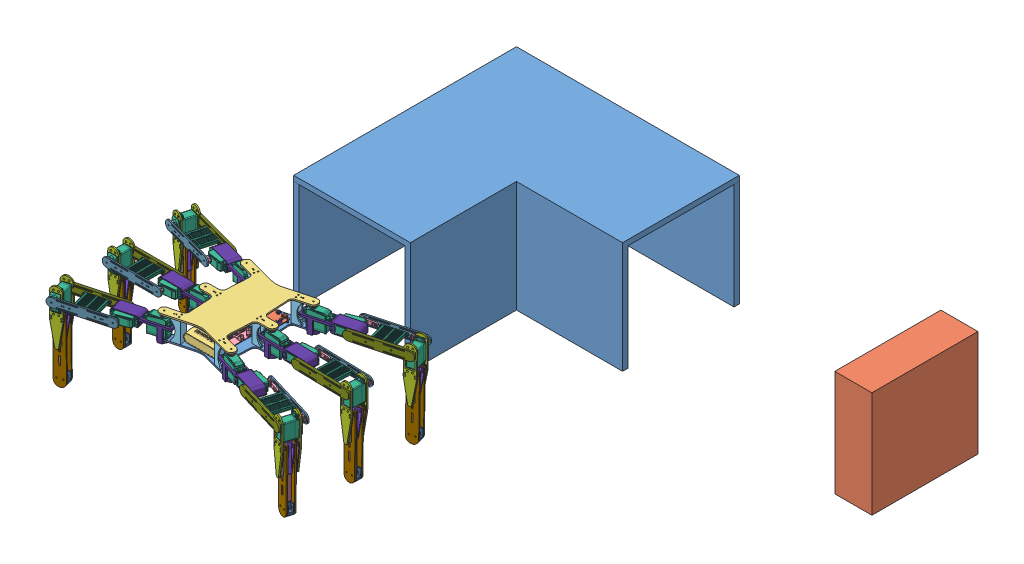
SolidWorks assembly ObstacleCourse, configuration Default. Lengths in mm.
Overall size (1281.29 282.9 1001.36).
210 component instances, 40 part files, 3 mates.
Components (placement in the parent):
- Tunnel-1: Tunnel [Default] at (-133.9096 207.5789 158.7477) x (0 0 1) z (-1 0 0) size (533.4 266.7 533.4)
- Wall-1: Wall [Default] at (894.7904 207.5789 425.4477) size (88.9 254 254)
- FullAssembly-1: FullAssembly [Default] at (-185.9141 155.1575 649.3406) size (590.09 222.09 384.76)
  - BodyAssembly-1: BodyAssembly [Default] at (93.0903 134.9257 147.182) size (181 51.83 218.31)
    - TopPlate-1: TopPlate [Default] at (90.5661 120.22 158.5049) size (181 3.17 218.31)
    - Aluminium 25T Servo Horn-1: Aluminium 25T Servo Horn [Default] at (10.5661 120.22 257.1595) x (0.965926 0 -0.258819) z (0 1 0) size (35.39 15.87 6)
    - Aluminium 25T Servo Horn-2: Aluminium 25T Servo Horn [Default] at (10.5661 120.22 158.5049) x (1 0 0) z (0 1 0) size (35.39 15.87 6)
    - Aluminium 25T Servo Horn-3: Aluminium 25T Servo Horn [Default] at (170.5661 120.22 257.1595) x (-0.965926 0 -0.258819) z (0 1 0) size (35.39 15.87 6)
    - Aluminium 25T Servo Horn-4: Aluminium 25T Servo Horn [Default] at (170.5661 120.22 59.8503) x (-0.965926 0 0.258819) z (0 1 0) size (35.39 15.87 6)
    - Aluminium 25T Servo Horn-5: Aluminium 25T Servo Horn [Default] at (170.5661 120.22 158.5049) x (-1 0 0) z (0 1 0) size (35.39 15.87 6)
    - Aluminium 25T Servo Horn-6: Aluminium 25T Servo Horn [Default] at (10.5661 120.22 59.8503) x (0.965926 0 0.258819) z (0 1 0) size (35.39 15.87 6)
    - BodyStandoff-1: BodyStandoff [Default] at (155.8504 117.045 74.4774) x (-0.965926 0 0.258819) z (0 -1 0) size (20 20.64 48.65)
    - BodyStandoff-2: BodyStandoff [Default] at (28.5661 117.045 148.1849) x (1 0 0) z (0 -1 0) size (20 20.64 48.65)
    - BodyStandoff-3: BodyStandoff [Default] at (152.5661 117.045 168.8249) x (-1 0 0) z (0 -1 0) size (20 20.64 48.65)
    - BodyStandoff-4: BodyStandoff [Default] at (150.5084 117.045 262.4691) x (-0.965926 0 -0.258819) z (0 -1 0) size (20 20.64 48.65)
    - BodyStandoff-5: BodyStandoff [Default] at (30.6238 117.045 54.5407) x (0.965926 0 0.258819) z (0 -1 0) size (20 20.64 48.65)
    - BodyStandoff-6: BodyStandoff [Default] at (25.2817 117.045 242.5324) x (0.965926 0 -0.258819) z (0 -1 0) size (20 20.64 48.65)
  - LegAssembly-1: LegAssembly [Default] at (68.7155 20.3576 359.6903) x (0.267323 -0.008627 0.963568) z (-0.963568 -0.011394 0.267221) size (60.68 215.89 234.68)
    - LowerLegAssembly-1: LowerLegAssembly [Default] at (27.0721 179.3541 216.2254) x (-0.008726 0.999962 -0.000076) z (0.008727 0 -0.999962) size (214.1 48.83 26)
      - 20kg Servo-1: 20kg Servo [Default] at (19.931 7.4761 41.5788) size (55.1 45.65 20.12)
      - KneeFrontPlate-1: KneeFrontPlate [Default] at (40.481 40.4761 41.5788) x (0 0 1) z (-1 0 0) size (26 3.17 130.1)
      - KneeFrontPlate-2: KneeFrontPlate [Default] at (40.481 4.3011 41.5788) x (0 0 1) z (-1 0 0) size (26 3.17 130.1)
      - LowerLegMiddleStandoff-1: LowerLegMiddleStandoff [Default] at (-7.619 28.6386 34.2851) x (0 0 1) z (-1 0 0) size (11.41 13.32 68)
      - LowerLegMiddleStandoff-2: LowerLegMiddleStandoff [Default] at (-7.619 19.3136 48.8726) x (0 0 -1) z (-1 0 0) size (11.41 13.32 68)
      - LowerLegPlate-1: LowerLegPlate [Default] at (-7.619 30.6386 43.1663) x (0 0 1) z (-1 0 0) size (26 3.17 153)
      - LowerLegPlate-2: LowerLegPlate [Default] at (-7.619 14.1386 43.1663) x (0 0 1) z (-1 0 0) size (26 3.17 153)
      - Foot-1: Foot [Default] at (-142.619 28.6436 41.5788) x (0 0 1) z (-1 0 0) size (26 13.33 28)
      - LowerLegSideStandoff-1: LowerLegSideStandoff [Default] at (-7.619 38.4761 34.2851) x (0 0 1) z (-1 0 0) size (11.41 6.66 68)
      - LowerLegSideStandoff-4: LowerLegSideStandoff [Default] at (-7.619 9.4761 48.8726) x (0 0 -1) z (-1 0 0) size (11.41 6.66 68)
      - MirrorLowerLegSideStandoff-10: MirrorLowerLegSideStandoff [Default] at (-7.619 9.4761 34.2851) x (0 0 1) z (1 0 0) size (11.41 6.66 68)
      - MirrorLowerLegSideStandoff-11: MirrorLowerLegSideStandoff [Default] at (-7.619 38.4761 48.8726) x (0 0 -1) z (1 0 0) size (11.41 6.66 68)
      - LowerLegBone-1: LowerLegBone [Default] at (-7.619 23.9761 43.1663) x (0 1 0) z (-1 0 0) size (33 3.17 135)
    - UpperLegAssembly-1: UpperLegAssembly [Default] at (52.8994 191.2742 177.6224) x (0.008825 -0.011318 -0.999897) z (0.999924 0.008727 0.008726) size (231.45 53.65 58.17)
      - Aluminium 25T Servo Horn-1: Aluminium 25T Servo Horn [Default] at (2.5459 18.2137 30.5337) size (35.39 15.87 6)
      - UpperLegFront-1: UpperLegFront [Default] at (2.5459 18.2137 33.7087) x (0 -1 0) z (1 0 0) size (21 3.17 141)
      - Aluminium 25T Servo Horn-2: Aluminium 25T Servo Horn [Default] at (122.5459 18.2137 30.5337) x (-1 0 0) z (0 0 1) size (35.39 15.87 6)
      - 20kg Servo-1: 20kg Servo [Default] at (132.4959 18.2137 -18.1163) x (-1 0 0) z (0 1 0) size (55.1 45.65 20.12)
      - UpperLegStandoff-1: UpperLegStandoff [Default] at (37.6959 18.2137 -18.1163) x (0 1 0) z (1 0 0) size (6 48.65 56)
      - UpperLegBack-1: UpperLegBack [Default] at (2.5459 18.2137 -18.1163) x (0 -1 0) z (1 0 0) size (21 3.17 141)
      - ShoulderMount-1: ShoulderMount [Default] at (102.5459 27.8363 -18.1163) x (1 0 0) z (0 -1 0) size (120 28.35 40.35)
      - 20kg Servo-2: 20kg Servo [Default] at (191.5459 -2.6363 -3.9413) size (55.1 45.65 20.12)
      - UpperLegBack-2: UpperLegBack [Default] at (2.5459 18.2137 -21.2913) x (0 -1 0) z (1 0 0) size (21 3.17 141)
    - Bearing-1: Bearing [Default] at (50.8194 178.3353 -22.7661) x (-0.059991 -0.011892 -0.998128) z (0.998162 0.007927 -0.060087) size (16 5 16)
  - LegAssembly-2: LegAssembly [Default] at (81.4626 20.3576 253.5138) x (0.008825 -0.008627 0.999924) z (-0.999897 -0.011394 0.008726) size (60.68 215.89 234.68)
    - LowerLegAssembly-1: LowerLegAssembly [Default] at (27.0721 179.3541 216.2254) x (-0.008726 0.999962 -0.000076) z (0.008727 0 -0.999962) size (214.1 48.83 26)
      - 20kg Servo-1: 20kg Servo [Default] at (19.931 7.4761 41.5788) size (55.1 45.65 20.12)
      - KneeFrontPlate-1: KneeFrontPlate [Default] at (40.481 40.4761 41.5788) x (0 0 1) z (-1 0 0) size (26 3.17 130.1)
      - KneeFrontPlate-2: KneeFrontPlate [Default] at (40.481 4.3011 41.5788) x (0 0 1) z (-1 0 0) size (26 3.17 130.1)
      - LowerLegMiddleStandoff-1: LowerLegMiddleStandoff [Default] at (-7.619 28.6386 34.2851) x (0 0 1) z (-1 0 0) size (11.41 13.32 68)
      - LowerLegMiddleStandoff-2: LowerLegMiddleStandoff [Default] at (-7.619 19.3136 48.8726) x (0 0 -1) z (-1 0 0) size (11.41 13.32 68)
      - LowerLegPlate-1: LowerLegPlate [Default] at (-7.619 30.6386 43.1663) x (0 0 1) z (-1 0 0) size (26 3.17 153)
      - LowerLegPlate-2: LowerLegPlate [Default] at (-7.619 14.1386 43.1663) x (0 0 1) z (-1 0 0) size (26 3.17 153)
      - Foot-1: Foot [Default] at (-142.619 28.6436 41.5788) x (0 0 1) z (-1 0 0) size (26 13.33 28)
      - LowerLegSideStandoff-1: LowerLegSideStandoff [Default] at (-7.619 38.4761 34.2851) x (0 0 1) z (-1 0 0) size (11.41 6.66 68)
      - LowerLegSideStandoff-4: LowerLegSideStandoff [Default] at (-7.619 9.4761 48.8726) x (0 0 -1) z (-1 0 0) size (11.41 6.66 68)
      - MirrorLowerLegSideStandoff-10: MirrorLowerLegSideStandoff [Default] at (-7.619 9.4761 34.2851) x (0 0 1) z (1 0 0) size (11.41 6.66 68)
      - MirrorLowerLegSideStandoff-11: MirrorLowerLegSideStandoff [Default] at (-7.619 38.4761 48.8726) x (0 0 -1) z (1 0 0) size (11.41 6.66 68)
      - LowerLegBone-1: LowerLegBone [Default] at (-7.619 23.9761 43.1663) x (0 1 0) z (-1 0 0) size (33 3.17 135)
    - UpperLegAssembly-1: UpperLegAssembly [Default] at (52.8994 191.2742 177.6224) x (0.008825 -0.011318 -0.999897) z (0.999924 0.008727 0.008726) size (231.45 53.65 58.17)
      - Aluminium 25T Servo Horn-1: Aluminium 25T Servo Horn [Default] at (2.5459 18.2137 30.5337) size (35.39 15.87 6)
      - UpperLegFront-1: UpperLegFront [Default] at (2.5459 18.2137 33.7087) x (0 -1 0) z (1 0 0) size (21 3.17 141)
      - Aluminium 25T Servo Horn-2: Aluminium 25T Servo Horn [Default] at (122.5459 18.2137 30.5337) x (-1 0 0) z (0 0 1) size (35.39 15.87 6)
      - 20kg Servo-1: 20kg Servo [Default] at (132.4959 18.2137 -18.1163) x (-1 0 0) z (0 1 0) size (55.1 45.65 20.12)
      - UpperLegStandoff-1: UpperLegStandoff [Default] at (37.6959 18.2137 -18.1163) x (0 1 0) z (1 0 0) size (6 48.65 56)
      - UpperLegBack-1: UpperLegBack [Default] at (2.5459 18.2137 -18.1163) x (0 -1 0) z (1 0 0) size (21 3.17 141)
      - ShoulderMount-1: ShoulderMount [Default] at (102.5459 27.8363 -18.1163) x (1 0 0) z (0 -1 0) size (120 28.35 40.35)
      - 20kg Servo-2: 20kg Servo [Default] at (191.5459 -2.6363 -3.9413) size (55.1 45.65 20.12)
      - UpperLegBack-2: UpperLegBack [Default] at (2.5459 18.2137 -21.2913) x (0 -1 0) z (1 0 0) size (21 3.17 141)
    - Bearing-1: Bearing [Default] at (50.8194 178.3353 -22.7661) x (-0.059991 -0.011892 -0.998128) z (0.998162 0.007927 -0.060087) size (16 5 16)
  - LegAssembly-3: LegAssembly [Default] at (95.7223 20.3576 150.8928) x (-0.250275 -0.008627 0.968136) z (-0.968085 -0.011394 -0.250364) size (60.68 215.89 234.68)
    - LowerLegAssembly-1: LowerLegAssembly [Default] at (27.0721 179.3541 216.2254) x (-0.008726 0.999962 -0.000076) z (0.008727 0 -0.999962) size (214.1 48.83 26)
      - 20kg Servo-1: 20kg Servo [Default] at (19.931 7.4761 41.5788) size (55.1 45.65 20.12)
      - KneeFrontPlate-1: KneeFrontPlate [Default] at (40.481 40.4761 41.5788) x (0 0 1) z (-1 0 0) size (26 3.17 130.1)
      - KneeFrontPlate-2: KneeFrontPlate [Default] at (40.481 4.3011 41.5788) x (0 0 1) z (-1 0 0) size (26 3.17 130.1)
      - LowerLegMiddleStandoff-1: LowerLegMiddleStandoff [Default] at (-7.619 28.6386 34.2851) x (0 0 1) z (-1 0 0) size (11.41 13.32 68)
      - LowerLegMiddleStandoff-2: LowerLegMiddleStandoff [Default] at (-7.619 19.3136 48.8726) x (0 0 -1) z (-1 0 0) size (11.41 13.32 68)
      - LowerLegPlate-1: LowerLegPlate [Default] at (-7.619 30.6386 43.1663) x (0 0 1) z (-1 0 0) size (26 3.17 153)
      - LowerLegPlate-2: LowerLegPlate [Default] at (-7.619 14.1386 43.1663) x (0 0 1) z (-1 0 0) size (26 3.17 153)
      - Foot-1: Foot [Default] at (-142.619 28.6436 41.5788) x (0 0 1) z (-1 0 0) size (26 13.33 28)
      - LowerLegSideStandoff-1: LowerLegSideStandoff [Default] at (-7.619 38.4761 34.2851) x (0 0 1) z (-1 0 0) size (11.41 6.66 68)
      - LowerLegSideStandoff-4: LowerLegSideStandoff [Default] at (-7.619 9.4761 48.8726) x (0 0 -1) z (-1 0 0) size (11.41 6.66 68)
      - MirrorLowerLegSideStandoff-10: MirrorLowerLegSideStandoff [Default] at (-7.619 9.4761 34.2851) x (0 0 1) z (1 0 0) size (11.41 6.66 68)
      - MirrorLowerLegSideStandoff-11: MirrorLowerLegSideStandoff [Default] at (-7.619 38.4761 48.8726) x (0 0 -1) z (1 0 0) size (11.41 6.66 68)
      - LowerLegBone-1: LowerLegBone [Default] at (-7.619 23.9761 43.1663) x (0 1 0) z (-1 0 0) size (33 3.17 135)
    - UpperLegAssembly-1: UpperLegAssembly [Default] at (52.8994 191.2742 177.6224) x (0.008825 -0.011318 -0.999897) z (0.999924 0.008727 0.008726) size (231.45 53.65 58.17)
      - Aluminium 25T Servo Horn-1: Aluminium 25T Servo Horn [Default] at (2.5459 18.2137 30.5337) size (35.39 15.87 6)
      - UpperLegFront-1: UpperLegFront [Default] at (2.5459 18.2137 33.7087) x (0 -1 0) z (1 0 0) size (21 3.17 141)
      - Aluminium 25T Servo Horn-2: Aluminium 25T Servo Horn [Default] at (122.5459 18.2137 30.5337) x (-1 0 0) z (0 0 1) size (35.39 15.87 6)
      - 20kg Servo-1: 20kg Servo [Default] at (132.4959 18.2137 -18.1163) x (-1 0 0) z (0 1 0) size (55.1 45.65 20.12)
      - UpperLegStandoff-1: UpperLegStandoff [Default] at (37.6959 18.2137 -18.1163) x (0 1 0) z (1 0 0) size (6 48.65 56)
      - UpperLegBack-1: UpperLegBack [Default] at (2.5459 18.2137 -18.1163) x (0 -1 0) z (1 0 0) size (21 3.17 141)
      - ShoulderMount-1: ShoulderMount [Default] at (102.5459 27.8363 -18.1163) x (1 0 0) z (0 -1 0) size (120 28.35 40.35)
      - 20kg Servo-2: 20kg Servo [Default] at (191.5459 -2.6363 -3.9413) size (55.1 45.65 20.12)
      - UpperLegBack-2: UpperLegBack [Default] at (2.5459 18.2137 -21.2913) x (0 -1 0) z (1 0 0) size (21 3.17 141)
    - Bearing-1: Bearing [Default] at (50.8194 178.3353 -22.7661) x (-0.059991 -0.011892 -0.998128) z (0.998162 0.007927 -0.060087) size (16 5 16)
  - LegAssembly-4: LegAssembly [Default] at (269.8625 20.3576 460.6982) x (0.279891 -0.008627 -0.959993) z (0.959939 -0.011394 0.279977) size (60.68 215.89 234.68)
    - LowerLegAssembly-1: LowerLegAssembly [Default] at (27.0721 179.3541 216.2254) x (-0.008726 0.999962 -0.000076) z (0.008727 0 -0.999962) size (214.1 48.83 26)
      - 20kg Servo-1: 20kg Servo [Default] at (19.931 7.4761 41.5788) size (55.1 45.65 20.12)
      - KneeFrontPlate-1: KneeFrontPlate [Default] at (40.481 40.4761 41.5788) x (0 0 1) z (-1 0 0) size (26 3.17 130.1)
      - KneeFrontPlate-2: KneeFrontPlate [Default] at (40.481 4.3011 41.5788) x (0 0 1) z (-1 0 0) size (26 3.17 130.1)
      - LowerLegMiddleStandoff-1: LowerLegMiddleStandoff [Default] at (-7.619 28.6386 34.2851) x (0 0 1) z (-1 0 0) size (11.41 13.32 68)
      - LowerLegMiddleStandoff-2: LowerLegMiddleStandoff [Default] at (-7.619 19.3136 48.8726) x (0 0 -1) z (-1 0 0) size (11.41 13.32 68)
      - LowerLegPlate-1: LowerLegPlate [Default] at (-7.619 30.6386 43.1663) x (0 0 1) z (-1 0 0) size (26 3.17 153)
      - LowerLegPlate-2: LowerLegPlate [Default] at (-7.619 14.1386 43.1663) x (0 0 1) z (-1 0 0) size (26 3.17 153)
      - Foot-1: Foot [Default] at (-142.619 28.6436 41.5788) x (0 0 1) z (-1 0 0) size (26 13.33 28)
      - LowerLegSideStandoff-1: LowerLegSideStandoff [Default] at (-7.619 38.4761 34.2851) x (0 0 1) z (-1 0 0) size (11.41 6.66 68)
      - LowerLegSideStandoff-4: LowerLegSideStandoff [Default] at (-7.619 9.4761 48.8726) x (0 0 -1) z (-1 0 0) size (11.41 6.66 68)
      - MirrorLowerLegSideStandoff-10: MirrorLowerLegSideStandoff [Default] at (-7.619 9.4761 34.2851) x (0 0 1) z (1 0 0) size (11.41 6.66 68)
      - MirrorLowerLegSideStandoff-11: MirrorLowerLegSideStandoff [Default] at (-7.619 38.4761 48.8726) x (0 0 -1) z (1 0 0) size (11.41 6.66 68)
      - LowerLegBone-1: LowerLegBone [Default] at (-7.619 23.9761 43.1663) x (0 1 0) z (-1 0 0) size (33 3.17 135)
    - UpperLegAssembly-1: UpperLegAssembly [Default] at (52.8994 191.2742 177.6224) x (0.008825 -0.011318 -0.999897) z (0.999924 0.008727 0.008726) size (231.45 53.65 58.17)
      - Aluminium 25T Servo Horn-1: Aluminium 25T Servo Horn [Default] at (2.5459 18.2137 30.5337) size (35.39 15.87 6)
      - UpperLegFront-1: UpperLegFront [Default] at (2.5459 18.2137 33.7087) x (0 -1 0) z (1 0 0) size (21 3.17 141)
      - Aluminium 25T Servo Horn-2: Aluminium 25T Servo Horn [Default] at (122.5459 18.2137 30.5337) x (-1 0 0) z (0 0 1) size (35.39 15.87 6)
      - 20kg Servo-1: 20kg Servo [Default] at (132.4959 18.2137 -18.1163) x (-1 0 0) z (0 1 0) size (55.1 45.65 20.12)
      - UpperLegStandoff-1: UpperLegStandoff [Default] at (37.6959 18.2137 -18.1163) x (0 1 0) z (1 0 0) size (6 48.65 56)
      - UpperLegBack-1: UpperLegBack [Default] at (2.5459 18.2137 -18.1163) x (0 -1 0) z (1 0 0) size (21 3.17 141)
      - ShoulderMount-1: ShoulderMount [Default] at (102.5459 27.8363 -18.1163) x (1 0 0) z (0 -1 0) size (120 28.35 40.35)
      - 20kg Servo-2: 20kg Servo [Default] at (191.5459 -2.6363 -3.9413) size (55.1 45.65 20.12)
      - UpperLegBack-2: UpperLegBack [Default] at (2.5459 18.2137 -21.2913) x (0 -1 0) z (1 0 0) size (21 3.17 141)
    - Bearing-1: Bearing [Default] at (50.8194 178.3353 -22.7661) x (-0.059991 -0.011892 -0.998128) z (0.998162 0.007927 -0.060087) size (16 5 16)
  - LegAssembly-5: LegAssembly [Default] at (284.5268 20.3576 358.4033) x (0.016403 -0.008627 -0.999828) z (0.999799 -0.011394 0.016501) size (60.68 215.89 234.68)
    - LowerLegAssembly-1: LowerLegAssembly [Default] at (27.0721 179.3541 216.2254) x (-0.008726 0.999962 -0.000076) z (0.008727 0 -0.999962) size (214.1 48.83 26)
      - 20kg Servo-1: 20kg Servo [Default] at (19.931 7.4761 41.5788) size (55.1 45.65 20.12)
      - KneeFrontPlate-1: KneeFrontPlate [Default] at (40.481 40.4761 41.5788) x (0 0 1) z (-1 0 0) size (26 3.17 130.1)
      - KneeFrontPlate-2: KneeFrontPlate [Default] at (40.481 4.3011 41.5788) x (0 0 1) z (-1 0 0) size (26 3.17 130.1)
      - LowerLegMiddleStandoff-1: LowerLegMiddleStandoff [Default] at (-7.619 28.6386 34.2851) x (0 0 1) z (-1 0 0) size (11.41 13.32 68)
      - LowerLegMiddleStandoff-2: LowerLegMiddleStandoff [Default] at (-7.619 19.3136 48.8726) x (0 0 -1) z (-1 0 0) size (11.41 13.32 68)
      - LowerLegPlate-1: LowerLegPlate [Default] at (-7.619 30.6386 43.1663) x (0 0 1) z (-1 0 0) size (26 3.17 153)
      - LowerLegPlate-2: LowerLegPlate [Default] at (-7.619 14.1386 43.1663) x (0 0 1) z (-1 0 0) size (26 3.17 153)
      - Foot-1: Foot [Default] at (-142.619 28.6436 41.5788) x (0 0 1) z (-1 0 0) size (26 13.33 28)
      - LowerLegSideStandoff-1: LowerLegSideStandoff [Default] at (-7.619 38.4761 34.2851) x (0 0 1) z (-1 0 0) size (11.41 6.66 68)
      - LowerLegSideStandoff-4: LowerLegSideStandoff [Default] at (-7.619 9.4761 48.8726) x (0 0 -1) z (-1 0 0) size (11.41 6.66 68)
      - MirrorLowerLegSideStandoff-10: MirrorLowerLegSideStandoff [Default] at (-7.619 9.4761 34.2851) x (0 0 1) z (1 0 0) size (11.41 6.66 68)
      - MirrorLowerLegSideStandoff-11: MirrorLowerLegSideStandoff [Default] at (-7.619 38.4761 48.8726) x (0 0 -1) z (1 0 0) size (11.41 6.66 68)
      - LowerLegBone-1: LowerLegBone [Default] at (-7.619 23.9761 43.1663) x (0 1 0) z (-1 0 0) size (33 3.17 135)
    - UpperLegAssembly-1: UpperLegAssembly [Default] at (52.8994 191.2742 177.6224) x (0.008825 -0.011318 -0.999897) z (0.999924 0.008727 0.008726) size (231.45 53.65 58.17)
      - Aluminium 25T Servo Horn-1: Aluminium 25T Servo Horn [Default] at (2.5459 18.2137 30.5337) size (35.39 15.87 6)
      - UpperLegFront-1: UpperLegFront [Default] at (2.5459 18.2137 33.7087) x (0 -1 0) z (1 0 0) size (21 3.17 141)
      - Aluminium 25T Servo Horn-2: Aluminium 25T Servo Horn [Default] at (122.5459 18.2137 30.5337) x (-1 0 0) z (0 0 1) size (35.39 15.87 6)
      - 20kg Servo-1: 20kg Servo [Default] at (132.4959 18.2137 -18.1163) x (-1 0 0) z (0 1 0) size (55.1 45.65 20.12)
      - UpperLegStandoff-1: UpperLegStandoff [Default] at (37.6959 18.2137 -18.1163) x (0 1 0) z (1 0 0) size (6 48.65 56)
      - UpperLegBack-1: UpperLegBack [Default] at (2.5459 18.2137 -18.1163) x (0 -1 0) z (1 0 0) size (21 3.17 141)
      - ShoulderMount-1: ShoulderMount [Default] at (102.5459 27.8363 -18.1163) x (1 0 0) z (0 -1 0) size (120 28.35 40.35)
      - 20kg Servo-2: 20kg Servo [Default] at (191.5459 -2.6363 -3.9413) size (55.1 45.65 20.12)
      - UpperLegBack-2: UpperLegBack [Default] at (2.5459 18.2137 -21.2913) x (0 -1 0) z (1 0 0) size (21 3.17 141)
    - Bearing-1: Bearing [Default] at (50.8194 178.3353 -22.7661) x (-0.059991 -0.011892 -0.998128) z (0.998162 0.007927 -0.060087) size (16 5 16)
  - LegAssembly-6: LegAssembly [Default] at (298.5972 20.3576 251.6835) x (-0.267323 -0.008627 -0.963568) z (0.963568 -0.011394 -0.267221) size (60.68 215.89 234.68)
    - LowerLegAssembly-1: LowerLegAssembly [Default] at (27.0721 179.3541 216.2254) x (-0.008726 0.999962 -0.000076) z (0.008727 0 -0.999962) size (214.1 48.83 26)
      - 20kg Servo-1: 20kg Servo [Default] at (19.931 7.4761 41.5788) size (55.1 45.65 20.12)
      - KneeFrontPlate-1: KneeFrontPlate [Default] at (40.481 40.4761 41.5788) x (0 0 1) z (-1 0 0) size (26 3.17 130.1)
      - KneeFrontPlate-2: KneeFrontPlate [Default] at (40.481 4.3011 41.5788) x (0 0 1) z (-1 0 0) size (26 3.17 130.1)
      - LowerLegMiddleStandoff-1: LowerLegMiddleStandoff [Default] at (-7.619 28.6386 34.2851) x (0 0 1) z (-1 0 0) size (11.41 13.32 68)
      - LowerLegMiddleStandoff-2: LowerLegMiddleStandoff [Default] at (-7.619 19.3136 48.8726) x (0 0 -1) z (-1 0 0) size (11.41 13.32 68)
      - LowerLegPlate-1: LowerLegPlate [Default] at (-7.619 30.6386 43.1663) x (0 0 1) z (-1 0 0) size (26 3.17 153)
      - LowerLegPlate-2: LowerLegPlate [Default] at (-7.619 14.1386 43.1663) x (0 0 1) z (-1 0 0) size (26 3.17 153)
      - Foot-1: Foot [Default] at (-142.619 28.6436 41.5788) x (0 0 1) z (-1 0 0) size (26 13.33 28)
      - LowerLegSideStandoff-1: LowerLegSideStandoff [Default] at (-7.619 38.4761 34.2851) x (0 0 1) z (-1 0 0) size (11.41 6.66 68)
      - LowerLegSideStandoff-4: LowerLegSideStandoff [Default] at (-7.619 9.4761 48.8726) x (0 0 -1) z (-1 0 0) size (11.41 6.66 68)
      - MirrorLowerLegSideStandoff-10: MirrorLowerLegSideStandoff [Default] at (-7.619 9.4761 34.2851) x (0 0 1) z (1 0 0) size (11.41 6.66 68)
      - MirrorLowerLegSideStandoff-11: MirrorLowerLegSideStandoff [Default] at (-7.619 38.4761 48.8726) x (0 0 -1) z (1 0 0) size (11.41 6.66 68)
      - LowerLegBone-1: LowerLegBone [Default] at (-7.619 23.9761 43.1663) x (0 1 0) z (-1 0 0) size (33 3.17 135)
    - UpperLegAssembly-1: UpperLegAssembly [Default] at (52.8994 191.2742 177.6224) x (0.008825 -0.011318 -0.999897) z (0.999924 0.008727 0.008726) size (231.45 53.65 58.17)
      - Aluminium 25T Servo Horn-1: Aluminium 25T Servo Horn [Default] at (2.5459 18.2137 30.5337) size (35.39 15.87 6)
      - UpperLegFront-1: UpperLegFront [Default] at (2.5459 18.2137 33.7087) x (0 -1 0) z (1 0 0) size (21 3.17 141)
      - Aluminium 25T Servo Horn-2: Aluminium 25T Servo Horn [Default] at (122.5459 18.2137 30.5337) x (-1 0 0) z (0 0 1) size (35.39 15.87 6)
      - 20kg Servo-1: 20kg Servo [Default] at (132.4959 18.2137 -18.1163) x (-1 0 0) z (0 1 0) size (55.1 45.65 20.12)
      - UpperLegStandoff-1: UpperLegStandoff [Default] at (37.6959 18.2137 -18.1163) x (0 1 0) z (1 0 0) size (6 48.65 56)
      - UpperLegBack-1: UpperLegBack [Default] at (2.5459 18.2137 -18.1163) x (0 -1 0) z (1 0 0) size (21 3.17 141)
      - ShoulderMount-1: ShoulderMount [Default] at (102.5459 27.8363 -18.1163) x (1 0 0) z (0 -1 0) size (120 28.35 40.35)
      - 20kg Servo-2: 20kg Servo [Default] at (191.5459 -2.6363 -3.9413) size (55.1 45.65 20.12)
      - UpperLegBack-2: UpperLegBack [Default] at (2.5459 18.2137 -21.2913) x (0 -1 0) z (1 0 0) size (21 3.17 141)
    - Bearing-1: Bearing [Default] at (50.8194 178.3353 -22.7661) x (-0.059991 -0.011892 -0.998128) z (0.998162 0.007927 -0.060087) size (16 5 16)
  - BottomBodyAssembly-1: BottomBodyAssembly [Default] at (83.95 98.1347 141.7913) size (181 28.22 218.31)
    - BottomPlate-1: BottomPlate [Default] at (99.7063 105.186 163.8956) size (181 3.17 218.31)
    - Raspberry Pi 4 Model B-1: Raspberry Pi 4 Model B [Default] at (101.4563 115.161 112.7766) x (-1 0 0) z (0 0 -1) size (88.99 19.9 58.4)
      - PCB, RPi4ModelB-1: PCB, RPi4ModelB [Default] at origin size (85 1.6 56)
      - Broadcom BCM2711B0 CPU, RPi4ModelB-1: Broadcom BCM2711B0 CPU, RPi4ModelB [Default] at (-13.25 0.8 -4.5) size (15 2.3 15)
      - 2.54 mm DUPONT MALE PIN HEADER, POE, 2X2, RPi4ModelB-1: 2.54 mm DUPONT MALE PIN HEADER, POE, 2X2, RPi4ModelB [Default] at (19 0.8 -18.5) size (5.08 11.3 5.08)
      - 2.54 mm DUPONT MALE PIN HEADER, IO, 2X20, RPi4ModelB-1: 2.54 mm DUPONT MALE PIN HEADER, IO, 2X20, RPi4ModelB [Default] at (-10 0.8 -24.5) size (50.8 11.3 5.08)
      - Camera Connector, RPi4ModelB-1: Camera Connector, RPi4ModelB [Default] at (4 0.8 16.5) x (0 0 -1) z (1 0 0) size (22.4 5.68 5.07)
      - Microphone Plug, RPi4ModelB-1: Microphone Plug, RPi4ModelB [Default] at (11.5 0.8 21.65) size (7.23 7.55 15)
      - Display Connector, RPi4ModelB-1: Display Connector, RPi4ModelB [Default] at (-38.5 0.8 0) x (0 0 1) z (-1 0 0) size (22.4 5.68 5.07)
      - Gigabit Ethernet Port, RPi4ModelB-1: Gigabit Ethernet Port, RPi4ModelB [Default] at (45.5 7.55 -17.75) x (0 0 -1) z (1 0 0) size (16.2 17.24 21.64)
      - Female Micro HDMI Connector, RPi4ModelB-2: Female Micro HDMI Connector, RPi4ModelB [Default] at (-3 0.8 27.3875) size (6.5 3.51 7.5)
      - Female Micro HDMI Connector, RPi4ModelB-3: Female Micro HDMI Connector, RPi4ModelB [Default] at (-16.5 0.8 27.3875) size (6.5 3.51 7.5)
      - Female USB Type C Connector, RPi4ModelB-1: Female USB Type C Connector, RPi4ModelB [Default] at (-31.3 0.8 26.5419) size (8.94 3.96 7.9)
      - 2X USB3.0 PORTS, RPi4ModelB-2: 2X USB3.0 PORTS, RPi4ModelB [Default] at (37.07 0.8 1) size (17.47 19.41 15.68)
      - 91D77 D9WHV 778K, 4 GB LPDDR4 SDRAM, RPi4ModelB-1: 91D77 D9WHV 778K, 4 GB LPDDR4 SDRAM, RPi4ModelB [Default] at (2.25 0.8 -4.5) size (10 0.8 14.5)
      - Cypress CYW43455 Wireless Module Cover, RPi4ModelB-1: Cypress CYW43455 Wireless Module Cover, RPi4ModelB [Default] at (-30.5 0.8 -14.5) size (11 1.6 13)
      - SD Card Slot, RPi4ModelB-1: SD Card Slot, RPi4ModelB [Default] at (-35.3 -0.8 0) x (0 0 -1) z (-1 0 0) size (11.95 1.45 11.4)
      - VIA VL805 PCIe USB 3.0 controller, RPi4ModelB-1: VIA VL805 PCIe USB 3.0 controller, RPi4ModelB [Default] at (17.5 0.8 4) size (8.8 0.8 8.8)
      - 2X USB2.0 PORTS, RPi4ModelB-1: 2X USB2.0 PORTS, RPi4ModelB [Default] at (37.065 0.65 19) size (17.87 19.16 15.33)
      - Broadcom BCM54213PE Gigabit Ethernet Transceiver, RPi4ModelB-1: Broadcom BCM54213PE Gigabit Ethernet Transceiver, RPi4ModelB [Default] at (16.5 0.8 -10) size (6.8 1 6.8)
      - MxL7704 Universal PMIC, RPi4ModelB-1: MxL7704 Universal PMIC, RPi4ModelB [Default] at (-32.5 0.8 16) size (5.4 0.8 5.4)
    - Pi Standoff-1: Pi Standoff [Default] at (140.4563 108.361 137.2766) size (3.46 6 3)
    - Pi Standoff-2: Pi Standoff [Default] at (82.4563 108.361 88.2766) size (3.46 6 3)
    - Pi Standoff-3: Pi Standoff [Default] at (140.4563 108.361 88.2766) size (3.46 6 3)
    - Pi Standoff-4: Pi Standoff [Default] at (82.4563 108.361 137.2766) size (3.46 6 3)
    - Intel Realsense D435-1: Intel Realsense D435 [Default] at (99.7063 120.861 233.3484) x (-1 0 0) z (0 1 0) size (90.24 25 25.08)
    - PCA9685-1: PCA9685 [Default] at (80.5027 115.861 186.6823) x (0.003733 0 -0.999993) z (0.999993 0 0.003733) size (67.26 16.51 25.01)
    - Pi Standoff-5: Pi Standoff [Default] at (70.7063 108.361 214.8956) size (3.46 6 3)
    - Pi Standoff-6: Pi Standoff [Default] at (89.7063 108.361 158.8956) size (3.46 6 3)
    - Pi Standoff-7: Pi Standoff [Default] at (109.7063 108.361 214.8956) size (3.46 6 3)
    - Pi Standoff-8: Pi Standoff [Default] at (89.7063 108.361 214.8956) size (3.46 6 3)
    - Pi Standoff-9: Pi Standoff [Default] at (70.7063 108.361 158.8956) size (3.46 6 3)
    - Pi Standoff-10: Pi Standoff [Default] at (128.7063 108.361 214.8956) size (3.46 6 3)
    - Pi Standoff-11: Pi Standoff [Default] at (128.7063 108.361 158.8956) size (3.46 6 3)
    - Pi Standoff-12: Pi Standoff [Default] at (109.7063 108.361 158.8956) size (3.46 6 3)
    - PCA9685-2: PCA9685 [Default] at (119.669 115.861 187.2541) x (0.006587 0 -0.999978) z (0.999978 0 0.006587) size (67.26 16.51 25.01)
Mates (geometry in assembly coordinates):
- Coincident1: coincident aligned: plane of Tunnel-1 through (132.7904 461.5789 425.4477) normal (0 0 1); plane of Wall-1 through (983.6904 207.5789 425.4477) normal (0 0 1)
- Coincident2: coincident aligned: plane of Tunnel-1 through (-133.9096 207.5789 158.7477) normal (0 -1 0); plane of Wall-1 through (983.6904 207.5789 425.4477) normal (0 -1 0)
- Distance1: distance = 508 mm anti-aligned: plane of Tunnel-1 through (386.7904 461.5789 425.4477) normal (1 0 0); plane of Wall-1 through (894.7904 207.5789 425.4477) normal (-1 0 0)
